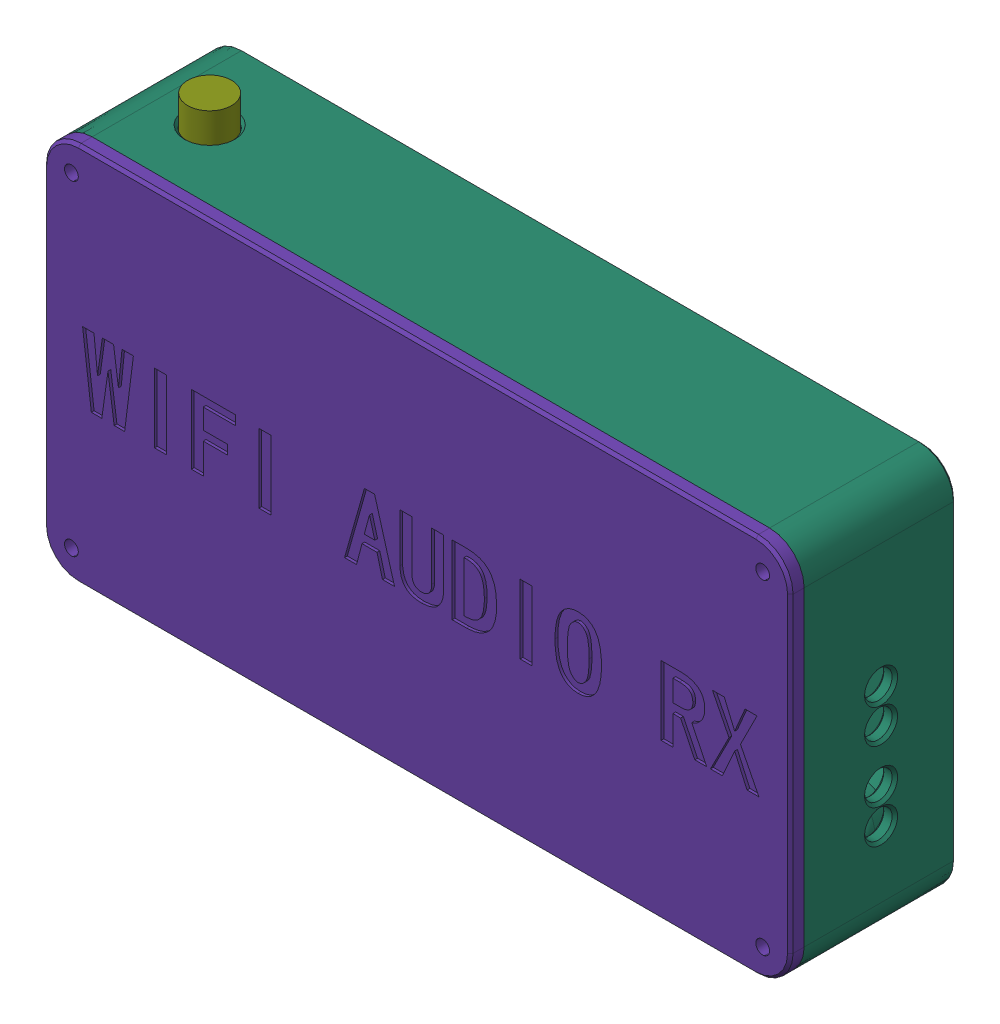
SolidWorks assembly WIFI-AUDIO-R, configuration 默认. Lengths in mm.
Overall size (108 59 24).
81 component instances, 17 part files, 9 mates.
Components (placement in the parent):
- 3D_WIFI-DSP_2025-06-08.step-1: 3D_WIFI-DSP_2025-06-08.step [默认] at (-57.684 19.7009 92.1932) size (96.75 36.93 14.51)
  - C50~C0603~C0603_L1.6-W0.8-H0.8~EbMB.step-1: C50~C0603~C0603_L1.6-W0.8-H0.8~EbMB.step [默认] at (41.7831 -8.509 1.6001) size (1.6 0.8 0.8)
    - C0603~C0603_L1.6-W0.8-H0.8~EbMB.step-1: C0603~C0603_L1.6-W0.8-H0.8~EbMB.step [默认] at origin size (1.6 0.8 0.8)
  - C50~C0603~C0603_L1.6-W0.8-H0.8~EbMB.step-2: C50~C0603~C0603_L1.6-W0.8-H0.8~EbMB.step [默认] at (55.7531 -26.5431 1.6001) size (1.6 0.8 0.8)
    - C0603~C0603_L1.6-W0.8-H0.8~EbMB.step-1: C0603~C0603_L1.6-W0.8-H0.8~EbMB.step [默认] at origin size (1.6 0.8 0.8)
  - C50~C0603~C0603_L1.6-W0.8-H0.8~EbMB.step-3: C50~C0603~C0603_L1.6-W0.8-H0.8~EbMB.step [默认] at (74.0411 -21.59 1.6001) size (1.6 0.8 0.8)
    - C0603~C0603_L1.6-W0.8-H0.8~EbMB.step-1: C0603~C0603_L1.6-W0.8-H0.8~EbMB.step [默认] at origin size (1.6 0.8 0.8)
  - C50~C0603~C0603_L1.6-W0.8-H0.8~EbMB.step-4: C50~C0603~C0603_L1.6-W0.8-H0.8~EbMB.step [默认] at (54.2291 -29.5911 1.6001) x (0 1 0) z (0 0 1) size (1.6 0.8 0.8)
    - C0603~C0603_L1.6-W0.8-H0.8~EbMB.step-1: C0603~C0603_L1.6-W0.8-H0.8~EbMB.step [默认] at origin size (1.6 0.8 0.8)
  - C50~C0603~C0603_L1.6-W0.8-H0.8~EbMB.step-5: C50~C0603~C0603_L1.6-W0.8-H0.8~EbMB.step [默认] at (56.3881 -29.5911 1.6001) x (0 1 0) z (0 0 1) size (1.6 0.8 0.8)
    - C0603~C0603_L1.6-W0.8-H0.8~EbMB.step-1: C0603~C0603_L1.6-W0.8-H0.8~EbMB.step [默认] at origin size (1.6 0.8 0.8)
  - C50~C0603~C0603_L1.6-W0.8-H0.8~EbMB.step-6: C50~C0603~C0603_L1.6-W0.8-H0.8~EbMB.step [默认] at (74.0411 -23.749 1.6001) size (1.6 0.8 0.8)
    - C0603~C0603_L1.6-W0.8-H0.8~EbMB.step-1: C0603~C0603_L1.6-W0.8-H0.8~EbMB.step [默认] at origin size (1.6 0.8 0.8)
  - C50~C0603~C0603_L1.6-W0.8-H0.8~EbMB.step-7: C50~C0603~C0603_L1.6-W0.8-H0.8~EbMB.step [默认] at (74.0411 -28.0671 1.6001) x (-1 0 0) z (0 0 1) size (1.6 0.8 0.8)
    - C0603~C0603_L1.6-W0.8-H0.8~EbMB.step-1: C0603~C0603_L1.6-W0.8-H0.8~EbMB.step [默认] at origin size (1.6 0.8 0.8)
  - C50~C0603~C0603_L1.6-W0.8-H0.8~EbMB.step-8: C50~C0603~C0603_L1.6-W0.8-H0.8~EbMB.step [默认] at (74.0411 -30.2261 1.6001) size (1.6 0.8 0.8)
    - C0603~C0603_L1.6-W0.8-H0.8~EbMB.step-1: C0603~C0603_L1.6-W0.8-H0.8~EbMB.step [默认] at origin size (1.6 0.8 0.8)
  - C50~C0603~C0603_L1.6-W0.8-H0.8~EbMB.step-9: C50~C0603~C0603_L1.6-W0.8-H0.8~EbMB.step [默认] at (74.0411 -34.5441 1.6001) size (1.6 0.8 0.8)
    - C0603~C0603_L1.6-W0.8-H0.8~EbMB.step-1: C0603~C0603_L1.6-W0.8-H0.8~EbMB.step [默认] at origin size (1.6 0.8 0.8)
  - C50~C0603~C0603_L1.6-W0.8-H0.8~EbMB.step-10: C50~C0603~C0603_L1.6-W0.8-H0.8~EbMB.step [默认] at (55.6261 -32.5121 1.6001) x (-1 0 0) z (0 0 1) size (1.6 0.8 0.8)
    - C0603~C0603_L1.6-W0.8-H0.8~EbMB.step-1: C0603~C0603_L1.6-W0.8-H0.8~EbMB.step [默认] at origin size (1.6 0.8 0.8)
  - C50~C0603~C0603_L1.6-W0.8-H0.8~EbMB.step-11: C50~C0603~C0603_L1.6-W0.8-H0.8~EbMB.step [默认] at (55.7531 -24.638 1.6001) x (-1 0 0) z (0 0 1) size (1.6 0.8 0.8)
    - C0603~C0603_L1.6-W0.8-H0.8~EbMB.step-1: C0603~C0603_L1.6-W0.8-H0.8~EbMB.step [默认] at origin size (1.6 0.8 0.8)
  - C50~C0603~C0603_L1.6-W0.8-H0.8~EbMB.step-12: C50~C0603~C0603_L1.6-W0.8-H0.8~EbMB.step [默认] at (74.0411 -25.9081 1.6001) x (-1 0 0) z (0 0 1) size (1.6 0.8 0.8)
    - C0603~C0603_L1.6-W0.8-H0.8~EbMB.step-1: C0603~C0603_L1.6-W0.8-H0.8~EbMB.step [默认] at origin size (1.6 0.8 0.8)
  - C50~C0603~C0603_L1.6-W0.8-H0.8~EbMB.step-13: C50~C0603~C0603_L1.6-W0.8-H0.8~EbMB.step [默认] at (74.0411 -32.3851 1.6001) x (-1 0 0) z (0 0 1) size (1.6 0.8 0.8)
    - C0603~C0603_L1.6-W0.8-H0.8~EbMB.step-1: C0603~C0603_L1.6-W0.8-H0.8~EbMB.step [默认] at origin size (1.6 0.8 0.8)
  - C50~C0603~C0603_L1.6-W0.8-H0.8~EbMB.step-14: C50~C0603~C0603_L1.6-W0.8-H0.8~EbMB.step [默认] at (42.5451 -2.413 1.6001) x (0 -1 0) z (0 0 1) size (1.6 0.8 0.8)
    - C0603~C0603_L1.6-W0.8-H0.8~EbMB.step-1: C0603~C0603_L1.6-W0.8-H0.8~EbMB.step [默认] at origin size (1.6 0.8 0.8)
  - U20~TO-263-3_L8.6-W10.2-P2.54-LS14.4-BR~TO-263-3_L10.2-W8.7-H4.5-LS14.4-P2.54~EbMB.step-1: U20~TO-263-3_L8.6-W10.2-P2.54-LS14.4-BR~TO-263-3_L10.2-W8.7-H4.5-LS14.4-P2.54~EbMB.step [默认] at (22.1456 -23.7253 1.6001) x (0 1 0) z (0 0 1) size (14.23 10.2 4.5)
    - TO-263-3_L8.6-W10.2-P2.54-LS14.4-BR~TO-263-3_L10.2-W8.7-H4.5-LS14.4-P2.54~EbMB.step-1: TO-263-3_L8.6-W10.2-P2.54-LS14.4-BR~TO-263-3_L10.2-W8.7-H4.5-LS14.4-P2.54~EbMB.step [默认] at origin size (14.23 10.2 4.5)
  - C107~C0805~C0805_L2.0-W1.3-H1.3~EbMB.step-1: C107~C0805~C0805_L2.0-W1.3-H1.3~EbMB.step [默认] at (91.013 -31.2499 1.6001) x (-1 0 0) z (0 0 1) size (2 1.3 1.3)
    - C0805~C0805_L2.0-W1.3-H1.3~EbMB.step-1: C0805~C0805_L2.0-W1.3-H1.3~EbMB.step [默认] at origin size (2 1.3 1.3)
  - C107~C0805~C0805_L2.0-W1.3-H1.3~EbMB.step-2: C107~C0805~C0805_L2.0-W1.3-H1.3~EbMB.step [默认] at (91.013 -22.9669 1.6001) x (-1 0 0) z (0 0 1) size (2 1.3 1.3)
    - C0805~C0805_L2.0-W1.3-H1.3~EbMB.step-1: C0805~C0805_L2.0-W1.3-H1.3~EbMB.step [默认] at origin size (2 1.3 1.3)
  - C107~C0805~C0805_L2.0-W1.3-H1.3~EbMB.step-3: C107~C0805~C0805_L2.0-W1.3-H1.3~EbMB.step [默认] at (91.013 -14.6838 1.6001) x (-1 0 0) z (0 0 1) size (2 1.3 1.3)
    - C0805~C0805_L2.0-W1.3-H1.3~EbMB.step-1: C0805~C0805_L2.0-W1.3-H1.3~EbMB.step [默认] at origin size (2 1.3 1.3)
  - C107~C0805~C0805_L2.0-W1.3-H1.3~EbMB.step-4: C107~C0805~C0805_L2.0-W1.3-H1.3~EbMB.step [默认] at (90.6782 -6.096 1.6001) size (2 1.3 1.3)
    - C0805~C0805_L2.0-W1.3-H1.3~EbMB.step-1: C0805~C0805_L2.0-W1.3-H1.3~EbMB.step [默认] at origin size (2 1.3 1.3)
  - SETTING0~CONN-TH_2P-P2.50_HX25003-2A~CONN-TH_2P-P2.50_HX25003-2A~EbMB.step-1: SETTING0~CONN-TH_2P-P2.50_HX25003-2A~CONN-TH_2P-P2.50_HX25003-2A~EbMB.step [默认] at (37.7191 -17.145 1.6001) size (7.5 5.9 10.6)
    - CONN-TH_2P-P2.50_HX25003-2A~CONN-TH_2P-P2.50_HX25003-2A~EbMB.step-1: CONN-TH_2P-P2.50_HX25003-2A~CONN-TH_2P-P2.50_HX25003-2A~EbMB.step [默认] at origin size (7.5 5.9 10.6)
  - C51~CAP-SMD_BD6.3-L6.6-W6.6-FD~CAP-SMD_BD6.3-L6.6-W6.6-FD~EbMB.step-1: C51~CAP-SMD_BD6.3-L6.6-W6.6-FD~CAP-SMD_BD6.3-L6.6-W6.6-FD~EbMB.step [默认] at (19.558 -7.112 1.6001) x (0 1 0) z (0 0 1) size (7.8 6.6 7.75)
    - CAP-SMD_BD6.3-L6.6-W6.6-FD~CAP-SMD_BD6.3-L6.6-W6.6-FD~EbMB.step-1: CAP-SMD_BD6.3-L6.6-W6.6-FD~CAP-SMD_BD6.3-L6.6-W6.6-FD~EbMB.step [默认] at origin size (7.8 6.6 7.75)
  - C51~CAP-SMD_BD6.3-L6.6-W6.6-FD~CAP-SMD_BD6.3-L6.6-W6.6-FD~EbMB.step-2: C51~CAP-SMD_BD6.3-L6.6-W6.6-FD~CAP-SMD_BD6.3-L6.6-W6.6-FD~EbMB.step [默认] at (27.3051 -11.176 1.6001) x (0 1 0) z (0 0 1) size (7.8 6.6 7.75)
    - CAP-SMD_BD6.3-L6.6-W6.6-FD~CAP-SMD_BD6.3-L6.6-W6.6-FD~EbMB.step-1: CAP-SMD_BD6.3-L6.6-W6.6-FD~CAP-SMD_BD6.3-L6.6-W6.6-FD~EbMB.step [默认] at origin size (7.8 6.6 7.75)
  - C51~CAP-SMD_BD6.3-L6.6-W6.6-FD~CAP-SMD_BD6.3-L6.6-W6.6-FD~EbMB.step-3: C51~CAP-SMD_BD6.3-L6.6-W6.6-FD~CAP-SMD_BD6.3-L6.6-W6.6-FD~EbMB.step [默认] at (47.8791 -32.3851 1.6001) x (-1 0 0) z (0 0 1) size (7.8 6.6 7.75)
    - CAP-SMD_BD6.3-L6.6-W6.6-FD~CAP-SMD_BD6.3-L6.6-W6.6-FD~EbMB.step-1: CAP-SMD_BD6.3-L6.6-W6.6-FD~CAP-SMD_BD6.3-L6.6-W6.6-FD~EbMB.step [默认] at origin size (7.8 6.6 7.75)
  - C51~CAP-SMD_BD6.3-L6.6-W6.6-FD~CAP-SMD_BD6.3-L6.6-W6.6-FD~EbMB.step-4: C51~CAP-SMD_BD6.3-L6.6-W6.6-FD~CAP-SMD_BD6.3-L6.6-W6.6-FD~EbMB.step [默认] at (36.3221 -4.826 1.6001) x (0 1 0) z (0 0 1) size (7.8 6.6 7.75)
    - CAP-SMD_BD6.3-L6.6-W6.6-FD~CAP-SMD_BD6.3-L6.6-W6.6-FD~EbMB.step-1: CAP-SMD_BD6.3-L6.6-W6.6-FD~CAP-SMD_BD6.3-L6.6-W6.6-FD~EbMB.step [默认] at origin size (7.8 6.6 7.75)
  - C111~CAP-SMD_BD10.0-L10.3-W10.3-LS11.0-FD~CAP-SMD_BD10.0-L10.3-W10.3-H10.2~EbMB.step-1: C111~CAP-SMD_BD10.0-L10.3-W10.3-LS11.0-FD~CAP-SMD_BD10.0-L10.3-W10.3-H10.2~EbMB.step [默认] at (37.0841 -28.1941 1.6001) x (-1 0 0) z (0 0 1) size (11.6 10.3 10.21)
    - CAP-SMD_BD10.0-L10.3-W10.3-LS11.0-FD~CAP-SMD_BD10.0-L10.3-W10.3-H10.2~EbMB.step-1: CAP-SMD_BD10.0-L10.3-W10.3-LS11.0-FD~CAP-SMD_BD10.0-L10.3-W10.3-H10.2~EbMB.step [默认] at origin size (11.6 10.3 10.21)
  - L1~IND-SMD_L7.3-W6.8~IND-SMD_L7.3-W6.8-H3.0~EbMB.step-1: L1~IND-SMD_L7.3-W6.8~IND-SMD_L7.3-W6.8-H3.0~EbMB.step [默认] at (82.9312 -14.3087 1.6001) size (7.42 6.8 3.05)
    - IND-SMD_L7.3-W6.8~IND-SMD_L7.3-W6.8-H3.0~EbMB.step-1: IND-SMD_L7.3-W6.8~IND-SMD_L7.3-W6.8-H3.0~EbMB.step [默认] at origin size (7.42 6.8 3.05)
  - L1~IND-SMD_L7.3-W6.8~IND-SMD_L7.3-W6.8-H3.0~EbMB.step-2: L1~IND-SMD_L7.3-W6.8~IND-SMD_L7.3-W6.8-H3.0~EbMB.step [默认] at (82.9312 -22.7754 1.6001) size (7.42 6.8 3.05)
    - IND-SMD_L7.3-W6.8~IND-SMD_L7.3-W6.8-H3.0~EbMB.step-1: IND-SMD_L7.3-W6.8~IND-SMD_L7.3-W6.8-H3.0~EbMB.step [默认] at origin size (7.42 6.8 3.05)
  - L1~IND-SMD_L7.3-W6.8~IND-SMD_L7.3-W6.8-H3.0~EbMB.step-3: L1~IND-SMD_L7.3-W6.8~IND-SMD_L7.3-W6.8-H3.0~EbMB.step [默认] at (82.9312 -31.2421 1.6001) size (7.42 6.8 3.05)
    - IND-SMD_L7.3-W6.8~IND-SMD_L7.3-W6.8-H3.0~EbMB.step-1: IND-SMD_L7.3-W6.8~IND-SMD_L7.3-W6.8-H3.0~EbMB.step [默认] at origin size (7.42 6.8 3.05)
  - L1~IND-SMD_L7.3-W6.8~IND-SMD_L7.3-W6.8-H3.0~EbMB.step-4: L1~IND-SMD_L7.3-W6.8~IND-SMD_L7.3-W6.8-H3.0~EbMB.step [默认] at (82.9312 -5.842 1.6001) size (7.42 6.8 3.05)
    - IND-SMD_L7.3-W6.8~IND-SMD_L7.3-W6.8-H3.0~EbMB.step-1: IND-SMD_L7.3-W6.8~IND-SMD_L7.3-W6.8-H3.0~EbMB.step [默认] at origin size (7.42 6.8 3.05)
  - U15~HTSSOP-32_L11.0-W6.1-P0.65-LS8.1-BL-EP-4~HTSSOP-32_L11.0-W6.1-P0.65-LS8.1-BL-EP-4~EbMB.step-1: U15~HTSSOP-32_L11.0-W6.1-P0.65-LS8.1-BL-EP-4~HTSSOP-32_L11.0-W6.1-P0.65-LS8.1-BL-EP-4~EbMB.step [默认] at (64.3891 -29.5911 1.6001) x (0 -1 0) z (0 0 1) size (11 8.1 1.16)
    - HTSSOP-32_L11.0-W6.1-P0.65-LS8.1-BL-EP-4~HTSSOP-32_L11.0-W6.1-P0.65-LS8.1-BL-EP-4~EbMB.step-1: HTSSOP-32_L11.0-W6.1-P0.65-LS8.1-BL-EP-4~HTSSOP-32_L11.0-W6.1-P0.65-LS8.1-BL-EP-4~EbMB.step [默认] at origin size (11 8.1 1.16)
  - U14~CONN-TH_5P-P2.50_ZX-XH2.54-5PZZ~CONN-TH_5P-P2.50_ZX-XH2.54-5PZZ~EbMB.step-1: U14~CONN-TH_5P-P2.50_ZX-XH2.54-5PZZ~CONN-TH_5P-P2.50_ZX-XH2.54-5PZZ~EbMB.step [默认] at (70.7391 -9.398 1.6001) x (0 -1 0) z (0 0 1) size (15 5.91 10.4)
    - CONN-TH_5P-P2.50_ZX-XH2.54-5PZZ~CONN-TH_5P-P2.50_ZX-XH2.54-5PZZ~EbMB.step-1: CONN-TH_5P-P2.50_ZX-XH2.54-5PZZ~CONN-TH_5P-P2.50_ZX-XH2.54-5PZZ~EbMB.step [默认] at origin size (15 5.91 10.4)
  - U24~WIFI-SMD_ESP32-WROOM-32UE~WIFI-SMD_L19.2-18.0-H3.2-ESP32-WROOM-32UE~EbMB.step-1: U24~WIFI-SMD_ESP32-WROOM-32UE~WIFI-SMD_L19.2-18.0-H3.2-ESP32-WROOM-32UE~EbMB.step [默认] at (56.2611 -9.779 1.6001) size (18 19.2 3.2)
    - WIFI-SMD_ESP32-WROOM-32UE~WIFI-SMD_L19.2-18.0-H3.2-ESP32-WROOM-32UE~EbMB.step-1: WIFI-SMD_ESP32-WROOM-32UE~WIFI-SMD_L19.2-18.0-H3.2-ESP32-WROOM-32UE~EbMB.step [默认] at origin size (18 19.2 3.2)
  - U9~CONN-TH_P5.00_KF301-5.0-2P~CONN-TH_P5.00_KF301-5.0-2P~EbMB.step-1: U9~CONN-TH_P5.00_KF301-5.0-2P~CONN-TH_P5.00_KF301-5.0-2P~EbMB.step [默认] at (100.2032 -11.938 1.6001) x (0 1 0) z (0 0 1) size (10.4 7.46 13.15)
    - CONN-TH_P5.00_KF301-5.0-2P~CONN-TH_P5.00_KF301-5.0-2P~EbMB.step-1: CONN-TH_P5.00_KF301-5.0-2P~CONN-TH_P5.00_KF301-5.0-2P~EbMB.step [默认] at origin size (10.4 7.46 13.15)
  - U9~CONN-TH_P5.00_KF301-5.0-2P~CONN-TH_P5.00_KF301-5.0-2P~EbMB.step-2: U9~CONN-TH_P5.00_KF301-5.0-2P~CONN-TH_P5.00_KF301-5.0-2P~EbMB.step [默认] at (100.2032 -24.511 1.6001) x (0 1 0) z (0 0 1) size (10.4 7.46 13.15)
    - CONN-TH_P5.00_KF301-5.0-2P~CONN-TH_P5.00_KF301-5.0-2P~EbMB.step-1: CONN-TH_P5.00_KF301-5.0-2P~CONN-TH_P5.00_KF301-5.0-2P~EbMB.step [默认] at origin size (10.4 7.46 13.15)
  - U9~CONN-TH_P5.00_KF301-5.0-2P~CONN-TH_P5.00_KF301-5.0-2P~EbMB.step-3: U9~CONN-TH_P5.00_KF301-5.0-2P~CONN-TH_P5.00_KF301-5.0-2P~EbMB.step [默认] at (10.922 -17.907 1.6001) x (0 -1 0) z (0 0 1) size (10.4 7.46 13.15)
    - CONN-TH_P5.00_KF301-5.0-2P~CONN-TH_P5.00_KF301-5.0-2P~EbMB.step-1: CONN-TH_P5.00_KF301-5.0-2P~CONN-TH_P5.00_KF301-5.0-2P~EbMB.step [默认] at origin size (10.4 7.46 13.15)
  - R32~R0603~R0603~EbMB.step-1: R32~R0603~R0603~EbMB.step [默认] at (42.5451 -5.842 1.6001) x (0 1 0) z (0 0 1) size (1.62 0.81 0.45)
    - R0603~R0603~EbMB.step-1: R0603~R0603~EbMB.step [默认] at origin size (1.62 0.81 0.45)
  - R32~R0603~R0603~EbMB.step-2: R32~R0603~R0603~EbMB.step [默认] at (41.7831 -11.176 1.6001) x (-1 0 0) z (0 0 1) size (1.62 0.81 0.45)
    - R0603~R0603~EbMB.step-1: R0603~R0603~EbMB.step [默认] at origin size (1.62 0.81 0.45)
  - RN3~RES-ARRAY-SMD_0603-8P-L3.2-W1.6-BL~R0603-8P_L3.2-W1.6-H0.6~EbMB.step-1: RN3~RES-ARRAY-SMD_0603-8P-L3.2-W1.6-BL~R0603-8P_L3.2-W1.6-H0.6~EbMB.step [默认] at (47.7521 -24.003 1.6001) x (-1 0 0) z (0 0 1) size (3.2 1.6 0.5)
    - RES-ARRAY-SMD_0603-8P-L3.2-W1.6-BL~R0603-8P_L3.2-W1.6-H0.6~EbMB.step-1: RES-ARRAY-SMD_0603-8P-L3.2-W1.6-BL~R0603-8P_L3.2-W1.6-H0.6~EbMB.step [默认] at origin size (3.2 1.6 0.5)
  - Board~EbMB.step-1: Board~EbMB.step [默认] at origin size (96.75 36.93 1.6)
- WIFI-AUDIO-R-BOX-1: WIFI-AUDIO-R-BOX [默认] at (-55.4323 -21.9895 85.1932) x (1 0 0) z (0 -1 0) size (108 22 55)
- sma座-1: sma座 [默认] at (-43.4323 31.0105 97.1932) size (10 36 10)
- WIFI-AUDIO-R-BOX1-1: WIFI-AUDIO-R-BOX1 [默认] at (-55.4323 -21.9895 107.1932) x (1 0 0) z (0 -1 0) size (108 2 55)
Mates (geometry in assembly coordinates):
- 距离1: distance = 5 mm anti-aligned: plane of WIFI-AUDIO-R-BOX-1 through (-55.4323 -21.9895 87.1932) normal (0 0 1); plane of 3D_WIFI-DSP_2025-06-08.step-1/Board~EbMB.step-1 through (-2.0579 1.4763 92.1932) normal (0 0 -1)
- 平行1: parallel aligned: plane of 3D_WIFI-DSP_2025-06-08.step-1/Board~EbMB.step-1 through (-50.4323 19.9422 92.1932) normal (0 1 0); plane of WIFI-AUDIO-R-BOX-1 through (-55.4323 33.0105 87.1932) normal (0 1 0)
- 距离2: distance = 5 mm: plane of WIFI-AUDIO-R-BOX-1 through (-55.4323 -21.9895 87.1932) normal (-1 0 0); line of 3D_WIFI-DSP_2025-06-08.step-1/Board~EbMB.step-1 through (-50.4323 -16.9895 93.7933) axis (0 1 0)
- 距离3: distance = 5 mm aligned: plane of WIFI-AUDIO-R-BOX-1 through (-55.4323 -21.9895 87.1932) normal (0 -1 0); plane of 3D_WIFI-DSP_2025-06-08.step-1/Board~EbMB.step-1 through (46.3165 -16.9895 92.1932) normal (0 -1 0)
- 同心1: concentric anti-aligned: cylinder of sma座-1 through (-43.4323 1.0105 97.1932) axis (0 1 0) radius 1; cylinder of WIFI-AUDIO-R-BOX-1 through (-43.4323 33.0105 97.1932) axis (0 -1 0) radius 3.25
- 重合5: coincident anti-aligned: plane of WIFI-AUDIO-R-BOX-1 through (50.5677 31.0105 107.1932) normal (0 -1 0); plane of sma座-1 through (-43.4323 31.0105 97.1932) normal (0 1 0)
- 重合6: coincident anti-aligned: plane of WIFI-AUDIO-R-BOX-1 through (-55.4323 -21.9895 107.1932) normal (0 0 1); plane of WIFI-AUDIO-R-BOX1-1 through (-50.4323 -16.9895 107.1932) normal (0 0 -1)
- 重合7: coincident aligned: plane of WIFI-AUDIO-R-BOX-1 through (-55.4323 -21.9895 87.1932) normal (-1 0 0); plane of WIFI-AUDIO-R-BOX1-1 through (-55.4323 -16.9895 109.1932) normal (-1 0 0)
- 重合8: coincident aligned: plane of WIFI-AUDIO-R-BOX-1 through (-55.4323 -21.9895 87.1932) normal (0 -1 0); plane of WIFI-AUDIO-R-BOX1-1 through (-50.4323 -21.9895 109.1932) normal (0 -1 0)
